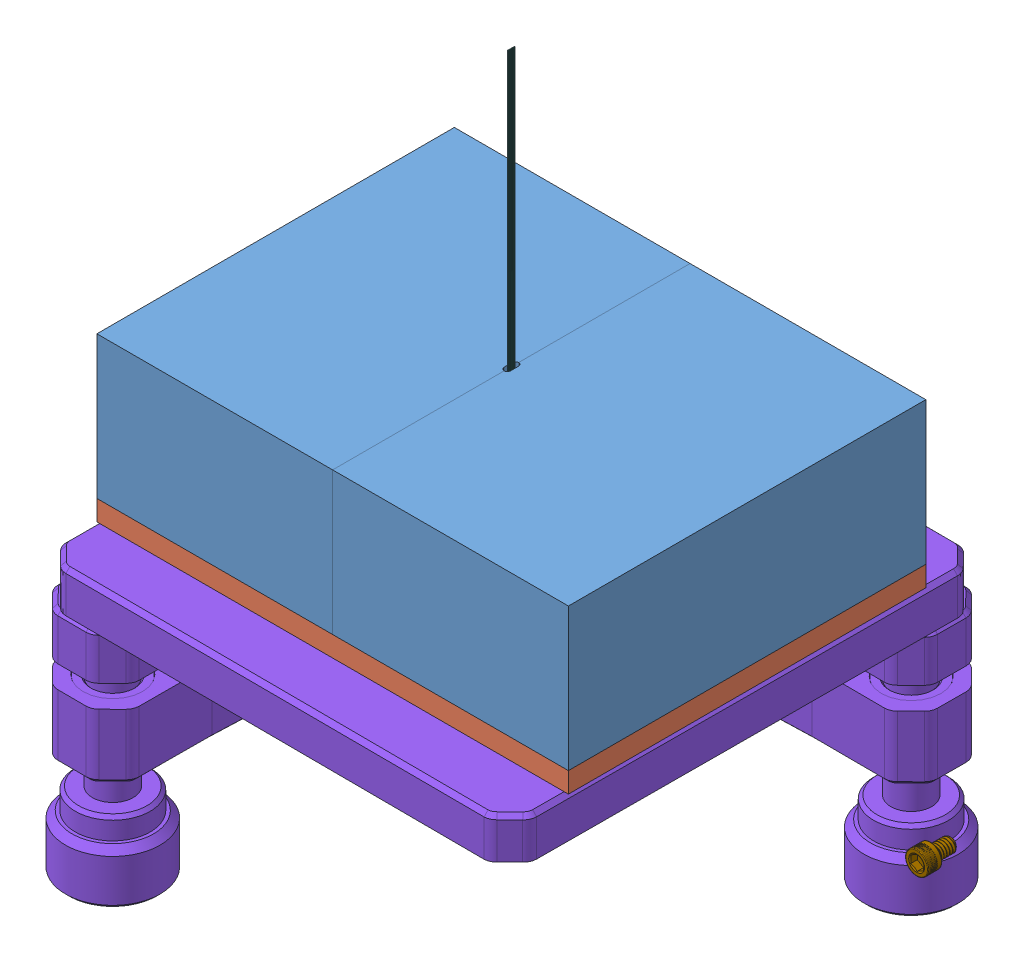
SolidWorks assembly Assembly, configuration Default. Lengths in mm.
Overall size (100.63 112.54 77.79).
15 component instances, 12 part files, 36 mates.
Components (placement in the parent):
- Box-1: Box [Default] at (46.9578 14.8481 6.1828) size (36.75 22.23 55.72)
- Lid-1: Lid [Default] at (10.2078 11.6731 6.1828) size (73.5 11 55.72)
- BeCu_Clamp-1: BeCu_Clamp [Default] at (46.9578 22.6731 25.4812) size (2.82 0.25 5.93)
- example_chip-2: example_chip [Default] at (42.0328 22.4231 28.9678) size (10 0.3 10)
- 92196A047_18-8 Stainless Steel Socket Head Screw-1: 92196A047_18-8 Stainless Steel Socket Head Screw [92196A047] at (46.9578 22.8954 25.4812) x (0.889022 0 -0.457865) z (0 1 0) size (2.44 2.44 3.27)
- 92196A047_18-8 Stainless Steel Socket Head Screw-2: 92196A047_18-8 Stainless Steel Socket Head Screw [92196A047] at (46.9578 22.8954 42.6044) x (0.945947 0 -0.32432) z (0 1 0) size (2.44 2.44 3.27)
- BeCu_Clamp-2: BeCu_Clamp [Default] at (46.9578 22.6731 42.6044) x (-1 0 0) z (0 0 -1) size (2.82 0.25 5.93)
- Fiber_Bundle-2: Fiber_Bundle [Default] at (45.7936 22.7231 35.2071) x (0 0 -1) z (1 0 0) size (2.48 57.1 2.48)
- Heater_Cart_02-1: Heater_Cart_02 [Default] at (34.2578 22.6731 11.1928) x (1 0 0) z (0 1 0) size (38.1 6.35 6.35)
- KM200B-Solidworks_edited-1: KM200B-Solidworks_edited [Default] at (7.5017 68.6543 -5.8381) x (0.999991 0 0.004196) z (0 -1 0) size (77.47 77.47 44.39)
- 91251A072_2-56_1_8th_Black-Oxide Alloy Steel Socket Head Screw-1: 91251A072_2-56_1_8th_Black-Oxide Alloy Steel Socket Head Screw [91251A072] at (106.0168 -2.4813 27.2472) size (3.57 3.57 5.6)
- Bottom_Block_off_plate-1: Bottom_Block_off_plate [Default] at (26.9228 9.6731 25.6928) size (40.07 2 16.7) (hidden)
- 380-025-213L001.step-1: 380-025-213L001.step [Default] at (18.4828 17.2231 34.0428) x (0 0 -1) z (0 1 0) size (29.7 7.35 10.8)
- micro-d-tes-aaray-4: micro-d-tes-aaray [Default] at (16.9578 22.6731 50.0428) x (0 0 -1) z (0 1 0) size (32 60 13.01)
- Box-2: Box [Default] at (46.9578 14.8481 61.9028) x (-1 0 0) z (0 0 -1) size (36.75 22.23 55.72)
Mates (geometry in assembly coordinates):
- Coincident1: coincident anti-aligned: plane of Box-1 through (46.9578 14.8481 6.1828) normal (0 -1 0); plane of Lid-1 through (10.2078 14.8481 6.1828) normal (0 1 0)
- Concentric4: concentric aligned: cylinder of Lid-1 through (62.9328 22.6731 14.3678) axis (0 1 0) radius 1.1303; circle of Heater_Cart_02-1
- Concentric5: concentric aligned: circle of Lid-1; circle of Heater_Cart_02-1
- Coincident2: coincident anti-aligned: plane of Lid-1 through (10.2078 22.6731 6.1828) normal (0 1 0); plane of Heater_Cart_02-1 through (34.2578 22.6731 11.1928) normal (0 -1 0)
- Concentric6: concentric anti-aligned: cylinder of BeCu_Clamp-1 through (46.9578 22.9271 25.4812) axis (0 -1 0) radius 0.8382; circle of 92196A047_18-8 Stainless Steel Socket Head Screw-1
- Coincident3: coincident anti-aligned: plane of BeCu_Clamp-1 through (46.9578 22.9271 25.4812) normal (0 1 0); plane of 92196A047_18-8 Stainless Steel Socket Head Screw-1 through (46.3996 22.9271 24.3973) normal (0 -1 0)
- Concentric7: concentric aligned: cylinder of Lid-1 through (46.9578 22.6731 25.4812) axis (0 1 0) radius 0.5956; circle of 92196A047_18-8 Stainless Steel Socket Head Screw-1
- Coincident4: coincident anti-aligned: plane of Lid-1 through (10.2078 22.6731 6.1828) normal (0 1 0); plane of BeCu_Clamp-1 through (46.9578 22.6731 25.4812) normal (0 -1 0)
- Concentric8: concentric aligned: cylinder of 92196A047_18-8 Stainless Steel Socket Head Screw-2 through (46.9578 21.3396 42.6044) axis (0 -1 0) radius 1.2192; cylinder of BeCu_Clamp-2 through (46.9578 22.9271 42.6044) axis (0 -1 0) radius 0.8382
- Coincident5: coincident anti-aligned: plane of 92196A047_18-8 Stainless Steel Socket Head Screw-2 through (46.5624 22.9271 41.4511) normal (0 -1 0); plane of BeCu_Clamp-2 through (46.9578 22.9271 42.6044) normal (0 1 0)
- Concentric9: concentric anti-aligned: cylinder of Lid-1 through (46.9578 22.6731 42.6044) axis (0 1 0) radius 0.5956; cylinder of 92196A047_18-8 Stainless Steel Socket Head Screw-2 through (46.9578 21.3396 42.6044) axis (0 -1 0) radius 1.2192
- Coincident6: coincident anti-aligned: plane of Lid-1 through (10.2078 22.6731 6.1828) normal (0 1 0); plane of BeCu_Clamp-2 through (46.9578 22.6731 42.6044) normal (0 -1 0)
- Parallel1: parallel aligned: plane of BeCu_Clamp-1 through (47.5801 22.9271 25.4812) normal (1 0 0); plane of BeCu_Clamp-2 through (47.5801 22.9271 42.6044) normal (1 0 0)
- Parallel2: parallel anti-aligned: plane of Lid-1 through (52.0328 22.4231 6.1828) normal (-1 0 0); plane of BeCu_Clamp-1 through (47.5801 22.9271 25.4812) normal (1 0 0)
- Concentric10: concentric: cylinder of Lid-1 through (64.9928 22.6731 34.0428) axis (0 -1 0) radius 1.7272; cylinder of KM200B-Solidworks_edited-1 through (64.9928 11.6731 34.0428) axis (0 1 0) radius 1.7272
- Parallel3: parallel: cylinder of Lid-1 through (28.9228 22.6731 34.0428) axis (0 -1 0) radius 1.7272; cylinder of KM200B-Solidworks_edited-1 through (28.9252 11.6731 33.8915) axis (0 1 0) radius 1.7272
- Coincident9: coincident anti-aligned: plane of Lid-1 through (10.2078 11.6731 6.1828) normal (0 -1 0); plane of Bottom_Block_off_plate-1 through (26.9228 11.6731 25.6928) normal (0 1 0)
- Coincident10: coincident anti-aligned: plane of Lid-1 through (52.0328 22.4231 6.1828) normal (-1 0 0); plane of example_chip-2 through (52.0328 22.7231 28.9678) normal (1 0 0)
- Coincident11: coincident anti-aligned: plane of Lid-1 through (10.2078 22.4231 28.9678) normal (0 0 1); plane of example_chip-2 through (42.0328 22.7231 28.9678) normal (0 0 -1)
- Coincident12: coincident anti-aligned: plane of Lid-1 through (41.8828 22.4231 28.9678) normal (0 1 0); plane of example_chip-2 through (42.0328 22.4231 28.9678) normal (0 -1 0)
- Concentric33: concentric aligned: cylinder of Lid-1 through (28.9228 11.6731 40.3928) axis (0 -1 0) radius 0.889; cylinder of Bottom_Block_off_plate-1 through (28.9228 11.6731 40.3928) axis (0 -1 0) radius 1.1303
- Concentric34: concentric aligned: cylinder of Lid-1 through (64.9928 11.6731 27.6928) axis (0 -1 0) radius 0.889; cylinder of Bottom_Block_off_plate-1 through (64.9928 11.6731 27.6928) axis (0 -1 0) radius 1.1303
- Concentric35: concentric anti-aligned: cylinder of Box-1 through (12.7078 14.8481 59.4028) axis (0 -1 0) radius 0.889; cylinder of Lid-1 through (12.7078 14.8481 59.4028) axis (0 1 0) radius 1.1303
- Concentric36: concentric aligned: cylinder of Lid-1 through (28.9578 22.6731 25.5428) axis (0 1 0) radius 0.889; cylinder of micro-d-tes-aaray-4 through (28.9578 21.8831 25.5428) axis (0 1 0) radius 1.15
- Concentric37: concentric aligned: circle of Lid-1; cylinder of micro-d-tes-aaray-4 through (64.9578 21.8831 25.5428) axis (0 1 0) radius 1.15
- Coincident22: coincident anti-aligned: plane of Lid-1 through (10.2078 22.6731 6.1828) normal (0 1 0); plane of micro-d-tes-aaray-4 through (46.9578 22.6731 34.0428) normal (0 -1 0)
- Coincident23: coincident anti-aligned: plane of example_chip-2 through (42.0328 22.7231 28.9678) normal (0 1 0); plane of Fiber_Bundle-2 through (45.7936 22.7231 35.2071) normal (0 -1 0)
- Parallel6: parallel anti-aligned: plane of Fiber_Bundle-2 through (48.2721 32.8231 35.2071) normal (1 0 0); plane of micro-d-tes-aaray-4 through (54.9578 22.6731 45.5428) normal (-1 0 0)
- Distance3: distance = 5 mm: point of Fiber_Bundle-2; line of example_chip-2 through (42.0328 22.7231 38.9678) axis (1 0 0)
- Distance4: distance = 5 mm: unknown of Fiber_Bundle-2; line of example_chip-2 through (52.0328 22.7231 38.9678) axis (0 0 -1)
- Concentric38: concentric: cylinder of Lid-1 through (64.9928 22.6731 34.0428) axis (0 -1 0) radius 1.7272; cylinder of KM200B-Solidworks_edited-1 through (64.9928 11.6731 34.0428) axis (0 1 0) radius 1.7272
- Parallel7: parallel: cylinder of Lid-1 through (28.9228 22.6731 34.0428) axis (0 -1 0) radius 1.7272; cylinder of KM200B-Solidworks_edited-1 through (28.9252 11.6731 33.8915) axis (0 1 0) radius 1.7272
- Coincident29: coincident anti-aligned: plane of Lid-1 through (10.2078 11.6731 6.1828) normal (0 -1 0); plane of KM200B-Solidworks_edited-1 through (79.7946 11.6731 -0.7087) normal (0 1 0)
- Concentric40: concentric: cylinder of Lid-1 through (56.9578 14.8481 59.4028) axis (0 1 0) radius 1.1303; cylinder of Box-2 through (56.9578 14.8481 59.4028) axis (0 -1 0) radius 0.889
- Concentric41: concentric: circle of Lid-1; cylinder of Box-2 through (56.9578 14.8481 8.6828) axis (0 -1 0) radius 0.889
- Coincident30: coincident anti-aligned: plane of Lid-1 through (10.2078 14.8481 6.1828) normal (0 1 0); plane of Box-2 through (46.9578 14.8481 61.9028) normal (0 -1 0)
